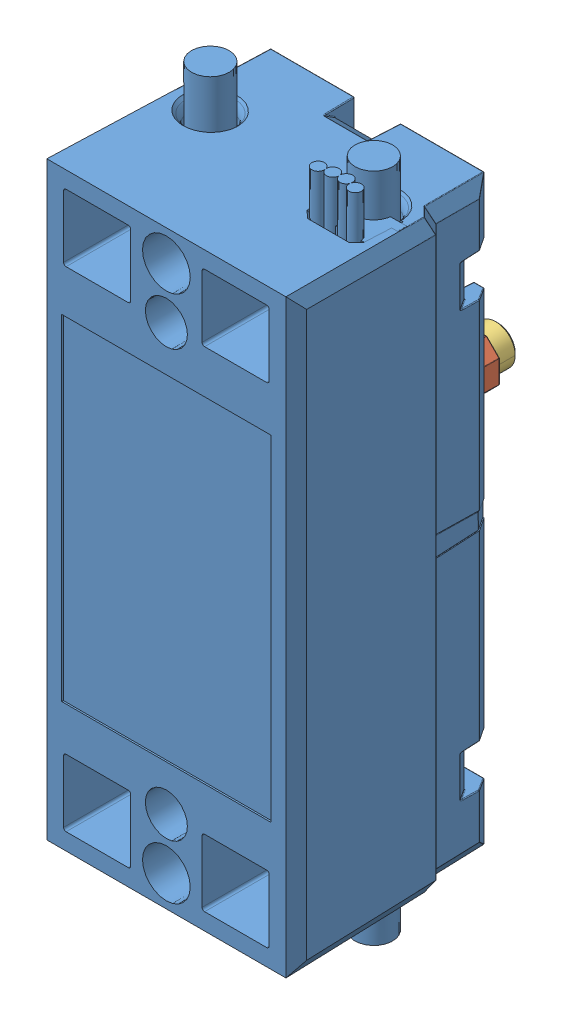
SolidWorks assembly Talon SRX (217-8080) (No Wires), configuration Default. Lengths in mm.
Overall size (30.47 80 30.05).
5 component instances, 3 part files, 0 mates.
Components (placement in the parent):
- Talon SRX (217-8080) (No Wires).step-1: Talon SRX (217-8080) (No Wires).step [Default] at origin size (30.47 80 30.05)
  - 217-8080-baseRev4_no wires.step-1: 217-8080-baseRev4_no wires.step [Default] at origin size (30.47 80 25.2)
  - 217-8080-002 Rev1.step-1: 217-8080-002 Rev1.step [Default] at (0 13.05 -9.65) x (1 0 0) z (0 -1 0) size (25.15 2.9 7.5)
  - 217-8080-005 Rev1_91251A105.step-1: 217-8080-005 Rev1_91251A105.step [Default] at (-9.525 13.05 -5.8875) size (4.65 4.65 7.61)
  - 217-8080-005 Rev1_91251A105.step-2: 217-8080-005 Rev1_91251A105.step [Default] at (9.525 13.05 -5.8875) size (4.65 4.65 7.61)
